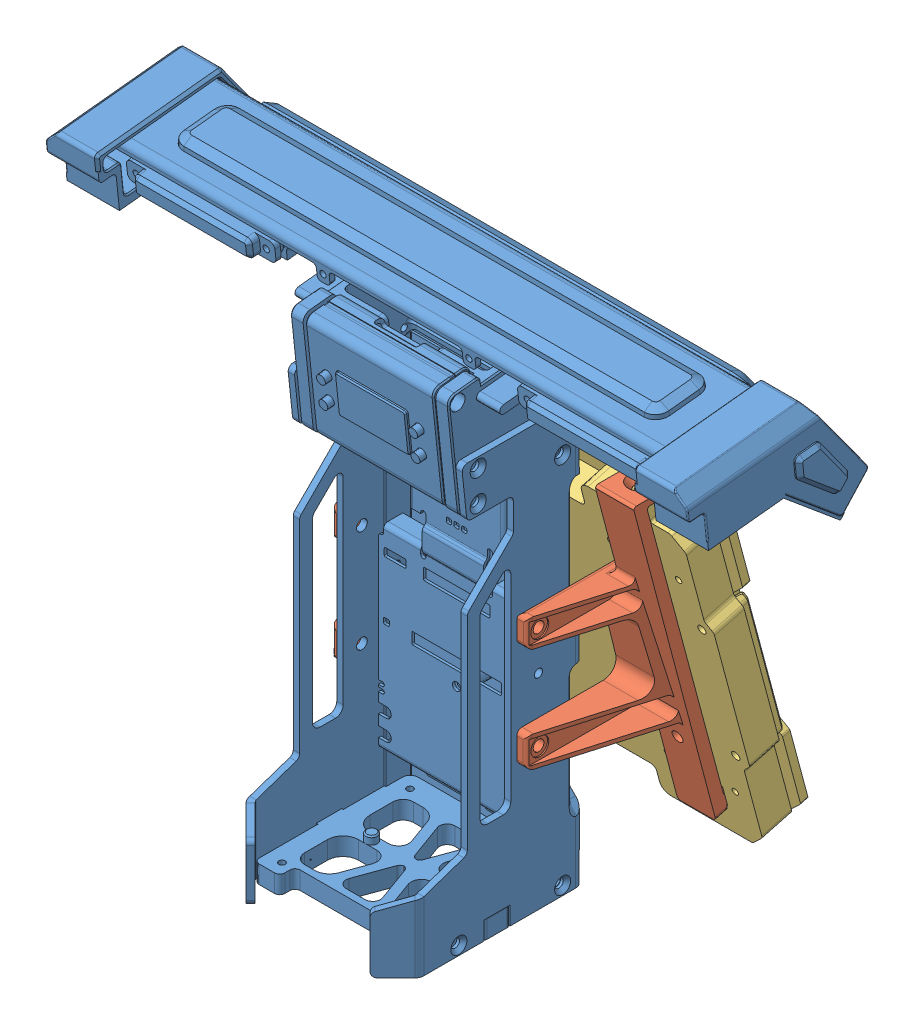
SolidWorks assembly 裁判系统血量柱带装甲, configuration 默认. Lengths in mm.
Overall size (254.6 207.47 130.58).
4 component instances, 4 part files, 9 mates.
Components (placement in the parent):
- 复件 裁判系统主控模块^裁判系统血量柱带装甲-1: 复件 裁判系统主控模块^裁判系统血量柱带装甲 [默认] at (18.2736 -91.1371 268.6546) size (254.6 207.47 93.71) (virtual)
- 复件 装甲支撑架（A）^裁判系统血量柱带装甲-1: 复件 装甲支撑架（A）^裁判系统血量柱带装甲 [默认] at (18.2736 -91.1371 268.6546) size (110 123.07 65.99) (virtual)
- 复件 小装甲^裁判系统血量柱带装甲-1: 复件 小装甲^裁判系统血量柱带装甲 [默认] at (18.2736 -91.1371 268.6546) size (141 126.74 52.99) (virtual)
- 复件 小装甲检测^裁判系统血量柱带装甲-1: 复件 小装甲检测^裁判系统血量柱带装甲 [默认] at (18.2736 -16.7969 188.5212) x (1 0 0) z (0 0.965926 0.258819) size (420.63 100 410.63) (hidden, virtual)
Mates (geometry in assembly coordinates):
- 重合1: coincident anti-aligned: plane of 复件 裁判系统主控模块^裁判系统血量柱带装甲-1 through (52.2736 73.8629 227.4546) normal (1 0 0); plane of 复件 装甲支撑架（A）^裁判系统血量柱带装甲-1 through (52.2736 13.5494 267.7785) normal (-1 0 0)
- 同心1: concentric aligned: cylinder of 复件 裁判系统主控模块^裁判系统血量柱带装甲-1 through (42.2736 7.8629 248.9203) axis (1 0 0) radius 2.1; cylinder of 复件 装甲支撑架（A）^裁判系统血量柱带装甲-1 through (47.5236 7.8629 248.9203) axis (1 0 0) radius 2.1
- 同心2: concentric aligned: cylinder of 复件 裁判系统主控模块^裁判系统血量柱带装甲-1 through (42.2736 -32.1371 248.9203) axis (1 0 0) radius 2.1; cylinder of 复件 装甲支撑架（A）^裁判系统血量柱带装甲-1 through (47.5236 -32.1371 248.9203) axis (1 0 0) radius 2.1
- 重合2: coincident anti-aligned: plane of 复件 装甲支撑架（A）^裁判系统血量柱带装甲-1 through (58.2736 44.7889 213.3053) normal (0 -1 0); plane of 复件 小装甲^裁判系统血量柱带装甲-1 through (58.2736 44.7889 224.1757) normal (0 1 0)
- 同心3: concentric aligned: cylinder of 复件 装甲支撑架（A）^裁判系统血量柱带装甲-1 through (65.7736 47.2889 219.2523) axis (0 1 0) radius 2.25; cylinder of 复件 小装甲^裁判系统血量柱带装甲-1 through (65.7736 44.7889 219.2523) axis (0 1 0) radius 1.65
- 重合3: coincident anti-aligned: plane of 复件 装甲支撑架（A）^裁判系统血量柱带装甲-1 through (65.7736 35.1741 221.5994) normal (0 0.258819 -0.965926); plane of 复件 小装甲^裁判系统血量柱带装甲-1 through (18.2736 -21.585 206.3908) normal (0 -0.258819 0.965926)
- 重合4: coincident anti-aligned: plane of 复件 小装甲^裁判系统血量柱带装甲-1 through (18.2736 -16.7969 188.5212) normal (0 0.258819 -0.965926); plane of 复件 小装甲检测^裁判系统血量柱带装甲-1 through (18.2736 -16.7969 188.5212) normal (0 -0.258819 0.965926)
- 宽度1: width aligned: plane of 复件 小装甲检测^裁判系统血量柱带装甲-1 through (85.7736 43.5735 204.6974) normal (0.573576 -0.212012 0.79124); plane of 复件 小装甲检测^裁判系统血量柱带装甲-1 through (-49.2264 43.5735 204.6974) normal (-0.573576 -0.212012 0.79124); plane of 复件 小装甲^裁判系统血量柱带装甲-1 through (-49.2264 -78.8496 178.6235) normal (-1 0 0); plane of 复件 小装甲^裁判系统血量柱带装甲-1 through (85.7736 -78.8496 178.6235) normal (1 0 0)
- 宽度2: width anti-aligned: plane of 复件 小装甲检测^裁判系统血量柱带装甲-1 through (-49.2264 43.5735 204.6974) normal (0 0.34202 0.939693); plane of 复件 小装甲检测^裁判系统血量柱带装甲-1 through (-49.2264 -77.1672 172.345) normal (0 -0.766044 0.642788); plane of 复件 小装甲^裁判系统血量柱带装甲-1 through (85.7736 43.5735 204.6974) normal (0 0.965926 0.258819); plane of 复件 小装甲^裁判系统血量柱带装甲-1 through (85.7736 -77.1672 172.345) normal (0 -0.965926 -0.258819)
